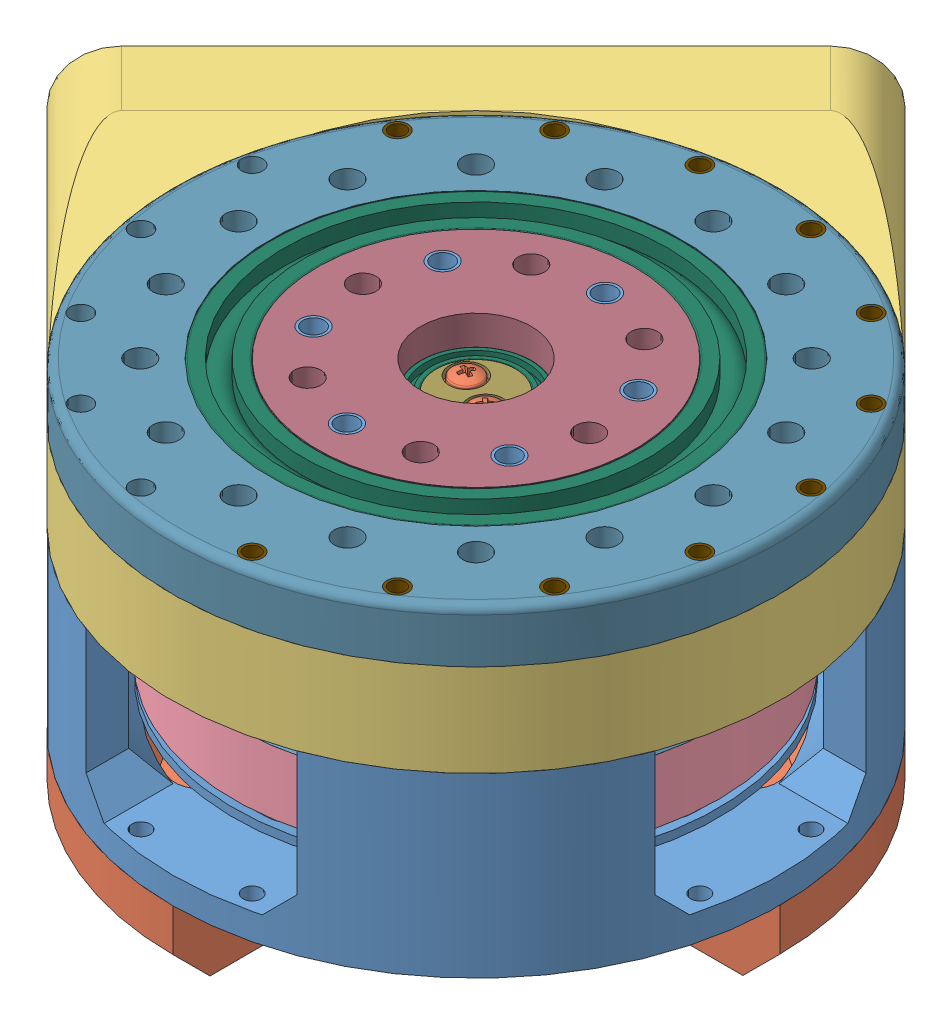
SolidWorks assembly Cycloidal_v2, configuration Default. Lengths in mm.
Overall size (173.24 87.5 173.24).
358 component instances, 93 part files, 154 mates.
Components (placement in the parent):
- motor-X83008S.stp-1: motor-X83008S.stp [Default] at (86.1463 89.8915 109.2516) x (-0.980342 0 -0.197304) z (0 -1 0) size (114.7 114.7 37.62)
  - base.stp-1: base.stp [Default] at (42.0794 12.0269 46.7342) size (91.6 91.6 15.61)
  - stator.stp-1: stator.stp [Default] at (42.0794 12.0269 33.1342) x (0.08493 -0.996387 0) z (0 0 1) size (83 83 8)
  - coil.stp-1: coil.stp [Default] at (39.5332 41.8984 37.1342) x (0.996387 0.08493 0) z (-0.08493 0.996387 0) size (4.4 10.2 10.5)
  - coil.stp-2: coil.stp [Default] at (34.3848 41.0025 37.1342) x (0.966502 0.256661 0) z (-0.256661 0.966502 0) size (4.4 10.2 10.5)
  - coil.stp-3: coil.stp [Default] at (29.4701 39.2261 37.1342) x (0.90725 0.420593 0) z (-0.420593 0.90725 0) size (4.4 10.2 10.5)
  - coil.stp-4: coil.stp [Default] at (24.9386 36.6233 37.1342) x (0.820431 0.571745 0) z (-0.571745 0.820431 0) size (4.4 10.2 10.5)
  - coil.stp-5: coil.stp [Default] at (20.9279 33.2732 37.1342) x (0.708685 0.705525 0) z (-0.705525 0.708685 0) size (4.4 10.2 10.5)
  - coil.stp-6: coil.stp [Default] at (17.5599 29.2775 37.1342) x (0.575405 0.817869 0) z (-0.817869 0.575405 0) size (4.4 10.2 10.5)
  - coil.stp-7: coil.stp [Default] at (14.9368 24.7576 37.1342) x (0.424642 0.905361 0) z (-0.905361 0.424642 0) size (4.4 10.2 10.5)
  - coil.stp-8: coil.stp [Default] at (13.1385 19.8509 37.1342) x (0.260976 0.965345 0) z (-0.965345 0.260976 0) size (4.4 10.2 10.5)
  - coil.stp-9: coil.stp [Default] at (12.2196 14.7066 37.1342) x (0.089381 0.995998 0) z (-0.995998 0.089381 0) size (4.4 10.2 10.5)
  - coil.stp-10: coil.stp [Default] at (12.2079 9.4807 37.1342) x (-0.08493 0.996387 0) z (-0.996387 -0.08493 0) size (4.4 10.2 10.5)
  - coil.stp-11: coil.stp [Default] at (13.1039 4.3323 37.1342) x (-0.256661 0.966502 0) z (-0.966502 -0.256661 0) size (4.4 10.2 10.5)
  - coil.stp-12: coil.stp [Default] at (14.8802 -0.5824 37.1342) x (-0.420593 0.90725 0) z (-0.90725 -0.420593 0) size (4.4 10.2 10.5)
  - coil.stp-13: coil.stp [Default] at (17.483 -5.1139 37.1342) x (-0.571745 0.820431 0) z (-0.820431 -0.571745 0) size (4.4 10.2 10.5)
  - coil.stp-14: coil.stp [Default] at (20.8332 -9.1246 37.1342) x (-0.705525 0.708685 0) z (-0.708685 -0.705525 0) size (4.4 10.2 10.5)
  - coil.stp-15: coil.stp [Default] at (24.8289 -12.4926 37.1342) x (-0.817869 0.575405 0) z (-0.575405 -0.817869 0) size (4.4 10.2 10.5)
  - coil.stp-16: coil.stp [Default] at (29.3487 -15.1157 37.1342) x (-0.905361 0.424642 0) z (-0.424642 -0.905361 0) size (4.4 10.2 10.5)
  - coil.stp-17: coil.stp [Default] at (34.2554 -16.914 37.1342) x (-0.965345 0.260976 0) z (-0.260976 -0.965345 0) size (4.4 10.2 10.5)
  - coil.stp-18: coil.stp [Default] at (39.3998 -17.8329 37.1342) x (-0.995998 0.089381 0) z (-0.089381 -0.995998 0) size (4.4 10.2 10.5)
  - coil.stp-19: coil.stp [Default] at (44.6256 -17.8446 37.1342) x (-0.996387 -0.08493 0) z (0.08493 -0.996387 0) size (4.4 10.2 10.5)
  - coil.stp-20: coil.stp [Default] at (49.7741 -16.9486 37.1342) x (-0.966502 -0.256661 0) z (0.256661 -0.966502 0) size (4.4 10.2 10.5)
  - coil.stp-21: coil.stp [Default] at (54.6887 -15.1723 37.1342) x (-0.90725 -0.420593 0) z (0.420593 -0.90725 0) size (4.4 10.2 10.5)
  - coil.stp-22: coil.stp [Default] at (59.2202 -12.5695 37.1342) x (-0.820431 -0.571745 0) z (0.571745 -0.820431 0) size (4.4 10.2 10.5)
  - coil.stp-23: coil.stp [Default] at (63.2309 -9.2193 37.1342) x (-0.708685 -0.705525 0) z (0.705525 -0.708685 0) size (4.4 10.2 10.5)
  - coil.stp-24: coil.stp [Default] at (66.599 -5.2236 37.1342) x (-0.575405 -0.817869 0) z (0.817869 -0.575405 0) size (4.4 10.2 10.5)
  - coil.stp-25: coil.stp [Default] at (69.222 -0.7038 37.1342) x (-0.424642 -0.905361 0) z (0.905361 -0.424642 0) size (4.4 10.2 10.5)
  - coil.stp-26: coil.stp [Default] at (71.0203 4.2029 37.1342) x (-0.260976 -0.965345 0) z (0.965345 -0.260976 0) size (4.4 10.2 10.5)
  - coil.stp-27: coil.stp [Default] at (71.9392 9.3473 37.1342) x (-0.089381 -0.995998 0) z (0.995998 -0.089381 0) size (4.4 10.2 10.5)
  - coil.stp-28: coil.stp [Default] at (71.9509 14.5731 37.1342) x (0.08493 -0.996387 0) z (0.996387 0.08493 0) size (4.4 10.2 10.5)
  - coil.stp-29: coil.stp [Default] at (71.055 19.7216 37.1342) x (0.256661 -0.966502 0) z (0.966502 0.256661 0) size (4.4 10.2 10.5)
  - coil.stp-30: coil.stp [Default] at (69.2786 24.6362 37.1342) x (0.420593 -0.90725 0) z (0.90725 0.420593 0) size (4.4 10.2 10.5)
  - coil.stp-31: coil.stp [Default] at (66.6758 29.1677 37.1342) x (0.571745 -0.820431 0) z (0.820431 0.571745 0) size (4.4 10.2 10.5)
  - coil.stp-32: coil.stp [Default] at (63.3257 33.1785 37.1342) x (0.705525 -0.708685 0) z (0.708685 0.705525 0) size (4.4 10.2 10.5)
  - coil.stp-33: coil.stp [Default] at (59.33 36.5465 37.1342) x (0.817869 -0.575405 0) z (0.575405 0.817869 0) size (4.4 10.2 10.5)
  - coil.stp-34: coil.stp [Default] at (54.8101 39.1695 37.1342) x (0.905361 -0.424642 0) z (0.424642 0.905361 0) size (4.4 10.2 10.5)
  - coil.stp-35: coil.stp [Default] at (49.9034 40.9678 37.1342) x (0.965345 -0.260976 0) z (0.260976 0.965345 0) size (4.4 10.2 10.5)
  - coil.stp-36: coil.stp [Default] at (44.759 41.8868 37.1342) x (0.995998 -0.089381 0) z (0.089381 0.995998 0) size (4.4 10.2 10.5)
  - rotor.stp-1: rotor.stp [Default] at (42.0794 12.0269 42.1342) x (-0.293442 0.955977 0) z (0 0 -1) size (91.8 91.8 12)
  - outrunner.stp-1: outrunner.stp [Default] at (42.0794 12.0269 30.1342) x (-0.254711 0.967017 0) z (-0.967017 -0.254711 0) size (91.8 17.01 91.8)
  - screw-mount.stp-1: screw-mount.stp [Default] at (38.1314 27.0157 27.1342) x (1 0 0) z (0 0 -1) size (7 7 6.5)
  - screw-mount.stp-2: screw-mount.stp [Default] at (27.0906 8.0789 27.1342) x (1 0 0) z (0 0 -1) size (7 7 6.5)
  - screw-mount.stp-3: screw-mount.stp [Default] at (57.0682 15.9749 27.1342) x (1 0 0) z (0 0 -1) size (7 7 6.5)
  - screw-mount.stp-4: screw-mount.stp [Default] at (46.0274 -2.9618 27.1342) x (1 0 0) z (0 0 -1) size (7 7 6.5)
  - 6702ZZ-bearing-15x21x4.stp-1: 6702ZZ-bearing-15x21x4.stp [Default] at (42.0794 12.0269 43.7342) x (1 0 0) z (0 -1 0) size (21 4 21)
  - 6702ZZ-bearing-15x21x4.stp-2: 6702ZZ-bearing-15x21x4.stp [Default] at (42.0794 12.0269 35.1342) x (1 0 0) z (0 1 0) size (21 4 21)
  - shaft.stp-1: shaft.stp [Default] at (42.0794 12.0269 20.1342) size (16 16 31.6)
  - fix-screw.stp-1: fix-screw.stp [Default] at (42.0794 12.0269 51.7342) x (1 0 0) z (0 0 -1) size (19.67 18.96 12.02)
- Base_Plate-1: Base_Plate [Default] at (47.267 69.7573 89.1587) x (0.897752 0 0.4405) z (-0.4405 0 0.897752) size (40 7 40)
- Eccentric_Shaft-1: Eccentric_Shaft [Default] at (31.2562 70.4165 89.8019) x (0.4405 0 -0.897752) z (0.897752 0 0.4405) size (20 15 17)
  - Eccentric_Shaft_bot-1: Eccentric_Shaft_bot [Default] at (7.6302 6.3409 14.0904) size (17 5 17)
  - Eccentric_Shaft_bot-2: Eccentric_Shaft_bot [Default] at (7.6302 11.3409 14.0904) x (-1 0 0) z (0 0 -1) size (17 5 17)
  - Eccentric_Shaft_top-1: Eccentric_Shaft_top [Default] at (7.6302 16.3409 14.0904) x (-1 0 0) z (0 0 -1) size (17 5 17)
- Output_Shaft-1: Output_Shaft [Default] at (47.267 87.2573 89.1587) x (-0.441786 0 -0.89712) z (0.89712 0 -0.441786) size (60 10 60)
- Cover-1: Cover [Default] at (47.267 87.2573 89.1587) x (0.707107 0 -0.707107) z (0.707107 0 0.707107) size (115 10.4 115)
- radial ball bearing_68_iso-39: radial ball bearing_68_iso [ISO 15 RBB - 1860 - 32,SI,NC,32_68] at (47.267 92.2573 89.1587) x (0 1 0) z (0 0 1) size (10 78 78)
- radial ball bearing_68_iso-40: radial ball bearing_68_iso [ISO 15 RBB - 1840 - 32,SI,NC,32_68] at (47.267 73.2573 89.1587) x (0 1 0) z (-0.019534 0 0.999809) size (7 52 52)
- m13_bearing-31: m13_bearing [Default] at (-10.7414 95.4081 67.0593) x (0.227678 0 0.973736) z (0.973736 0 -0.227678) size (13 16 13)
  - m6-1: m6 [Default] at (8.4921 2.5508 14.8914) size (6 16 6)
  - radial ball bearing_68_iso-1: radial ball bearing_68_iso [ISO 15 RBB - 286 - 10,SI,NC,10_68] at (8.4921 16.0508 14.8914) x (0 1 0) z (0 0 1) size (5 13 13)
  - radial ball bearing_68_iso-2: radial ball bearing_68_iso [ISO 15 RBB - 286 - 10,SI,NC,10_68] at (8.4921 11.0508 14.8914) x (0 1 0) z (0 0 1) size (5 13 13)
- m13_bearing-32: m13_bearing [Default] at (-14.1668 95.4081 84.2801) x (0.227678 0 0.973736) z (0.973736 0 -0.227678) size (13 16 13)
  - m6-1: m6 [Default] at (8.4921 2.5508 14.8914) size (6 16 6)
  - radial ball bearing_68_iso-1: radial ball bearing_68_iso [ISO 15 RBB - 286 - 10,SI,NC,10_68] at (8.4921 16.0508 14.8914) x (0 1 0) z (0 0 1) size (5 13 13)
  - radial ball bearing_68_iso-2: radial ball bearing_68_iso [ISO 15 RBB - 286 - 10,SI,NC,10_68] at (8.4921 11.0508 14.8914) x (0 1 0) z (0 0 1) size (5 13 13)
- m13_bearing-34: m13_bearing [Default] at (13.6125 95.5581 125.8547) x (0.227678 0 0.973736) z (0.973736 0 -0.227678) size (13 16 13)
  - m6-1: m6 [Default] at (8.4921 2.5508 14.8914) size (6 16 6)
  - radial ball bearing_68_iso-1: radial ball bearing_68_iso [ISO 15 RBB - 286 - 10,SI,NC,10_68] at (8.4921 16.0508 14.8914) x (0 1 0) z (0 0 1) size (5 13 13)
  - radial ball bearing_68_iso-2: radial ball bearing_68_iso [ISO 15 RBB - 286 - 10,SI,NC,10_68] at (8.4921 11.0508 14.8914) x (0 1 0) z (0 0 1) size (5 13 13)
- m13_bearing-35: m13_bearing [Default] at (-0.9866 95.4081 116.0999) x (0.227678 0 0.973736) z (0.973736 0 -0.227678) size (13 16 13)
  - m6-1: m6 [Default] at (8.4921 2.5508 14.8914) size (6 16 6)
  - radial ball bearing_68_iso-1: radial ball bearing_68_iso [ISO 15 RBB - 286 - 10,SI,NC,10_68] at (8.4921 16.0508 14.8914) x (0 1 0) z (0 0 1) size (5 13 13)
  - radial ball bearing_68_iso-2: radial ball bearing_68_iso [ISO 15 RBB - 286 - 10,SI,NC,10_68] at (8.4921 11.0508 14.8914) x (0 1 0) z (0 0 1) size (5 13 13)
- m13_bearing-36: m13_bearing [Default] at (-10.7414 95.5581 101.5009) x (0.227678 0 0.973736) z (0.973736 0 -0.227678) size (13 16 13)
  - m6-1: m6 [Default] at (8.4921 2.5508 14.8914) size (6 16 6)
  - radial ball bearing_68_iso-1: radial ball bearing_68_iso [ISO 15 RBB - 286 - 10,SI,NC,10_68] at (8.4921 16.0508 14.8914) x (0 1 0) z (0 0 1) size (5 13 13)
  - radial ball bearing_68_iso-2: radial ball bearing_68_iso [ISO 15 RBB - 286 - 10,SI,NC,10_68] at (8.4921 11.0508 14.8914) x (0 1 0) z (0 0 1) size (5 13 13)
- m13_bearing-1: m13_bearing [Default] at (-0.8801 95.4081 62.5627) x (0.736525 0 0.676411) z (0.676411 0 -0.736525) size (13 16 13)
  - m6-1: m6 [Default] at (8.4921 2.5508 14.8914) size (6 16 6)
  - radial ball bearing_68_iso-1: radial ball bearing_68_iso [ISO 15 RBB - 286 - 10,SI,NC,10_68] at (8.4921 16.0508 14.8914) x (0 1 0) z (0 0 1) size (5 13 13)
  - radial ball bearing_68_iso-2: radial ball bearing_68_iso [ISO 15 RBB - 286 - 10,SI,NC,10_68] at (8.4921 11.0508 14.8914) x (0 1 0) z (0 0 1) size (5 13 13)
- m13_bearing-2: m13_bearing [Default] at (48.6831 95.4081 124.0939) x (0.120271 0 0.992741) z (0.992741 0 -0.120271) size (13 16 13)
  - m6-1: m6 [Default] at (8.4921 2.5508 14.8914) size (6 16 6)
  - radial ball bearing_68_iso-1: radial ball bearing_68_iso [ISO 15 RBB - 286 - 10,SI,NC,10_68] at (8.4921 16.0508 14.8914) x (0 1 0) z (0 0 1) size (5 13 13)
  - radial ball bearing_68_iso-2: radial ball bearing_68_iso [ISO 15 RBB - 286 - 10,SI,NC,10_68] at (8.4921 11.0508 14.8914) x (0 1 0) z (0 0 1) size (5 13 13)
- m13_bearing-3: m13_bearing [Default] at (32.7832 95.4081 34.9886) x (-0.046141 0 0.998935) z (0.998935 0 0.046141) size (13 16 13)
  - m6-1: m6 [Default] at (8.4921 2.5508 14.8914) size (6 16 6)
  - radial ball bearing_68_iso-1: radial ball bearing_68_iso [ISO 15 RBB - 286 - 10,SI,NC,10_68] at (8.4921 16.0508 14.8914) x (0 1 0) z (0 0 1) size (5 13 13)
  - radial ball bearing_68_iso-2: radial ball bearing_68_iso [ISO 15 RBB - 286 - 10,SI,NC,10_68] at (8.4921 11.0508 14.8914) x (0 1 0) z (0 0 1) size (5 13 13)
- m13_bearing-4: m13_bearing [Default] at (77.1902 95.4081 81.0003) x (0.022268 0 0.999752) z (0.999752 0 -0.022268) size (13 16 13)
  - m6-1: m6 [Default] at (8.4921 2.5508 14.8914) size (6 16 6)
  - radial ball bearing_68_iso-1: radial ball bearing_68_iso [ISO 15 RBB - 286 - 10,SI,NC,10_68] at (8.4921 16.0508 14.8914) x (0 1 0) z (0 0 1) size (5 13 13)
  - radial ball bearing_68_iso-2: radial ball bearing_68_iso [ISO 15 RBB - 286 - 10,SI,NC,10_68] at (8.4921 11.0508 14.8914) x (0 1 0) z (0 0 1) size (5 13 13)
- m13_bearing-5: m13_bearing [Default] at (73.474 95.4081 98.7828) x (0.059133 0 0.99825) z (0.99825 0 -0.059133) size (13 16 13)
  - m6-1: m6 [Default] at (8.4921 2.5508 14.8914) size (6 16 6)
  - radial ball bearing_68_iso-1: radial ball bearing_68_iso [ISO 15 RBB - 286 - 10,SI,NC,10_68] at (8.4921 16.0508 14.8914) x (0 1 0) z (0 0 1) size (5 13 13)
  - radial ball bearing_68_iso-2: radial ball bearing_68_iso [ISO 15 RBB - 286 - 10,SI,NC,10_68] at (8.4921 11.0508 14.8914) x (0 1 0) z (0 0 1) size (5 13 13)
- m13_bearing-6: m13_bearing [Default] at (12.9248 95.4081 46.7315) x (0.451561 0 0.89224) z (0.89224 0 -0.451561) size (13 16 13)
  - m6-1: m6 [Default] at (8.4921 2.5508 14.8914) size (6 16 6)
  - radial ball bearing_68_iso-1: radial ball bearing_68_iso [ISO 15 RBB - 286 - 10,SI,NC,10_68] at (8.4921 16.0508 14.8914) x (0 1 0) z (0 0 1) size (5 13 13)
  - radial ball bearing_68_iso-2: radial ball bearing_68_iso [ISO 15 RBB - 286 - 10,SI,NC,10_68] at (8.4921 11.0508 14.8914) x (0 1 0) z (0 0 1) size (5 13 13)
- m13_bearing-7: m13_bearing [Default] at (56.6452 95.4081 32.3406) x (-0.545813 0 0.837907) z (0.837907 0 0.545813) size (13 16 13)
  - m6-1: m6 [Default] at (8.4921 2.5508 14.8914) size (6 16 6)
  - radial ball bearing_68_iso-1: radial ball bearing_68_iso [ISO 15 RBB - 286 - 10,SI,NC,10_68] at (8.4921 16.0508 14.8914) x (0 1 0) z (0 0 1) size (5 13 13)
  - radial ball bearing_68_iso-2: radial ball bearing_68_iso [ISO 15 RBB - 286 - 10,SI,NC,10_68] at (8.4921 11.0508 14.8914) x (0 1 0) z (0 0 1) size (5 13 13)
- m13_bearing-8: m13_bearing [Default] at (63.0373 95.4081 51.3153) x (0.158553 0 0.98735) z (0.98735 0 -0.158553) size (13 16 13)
  - m6-1: m6 [Default] at (8.4921 2.5508 14.8914) size (6 16 6)
  - radial ball bearing_68_iso-1: radial ball bearing_68_iso [ISO 15 RBB - 286 - 10,SI,NC,10_68] at (8.4921 16.0508 14.8914) x (0 1 0) z (0 0 1) size (5 13 13)
  - radial ball bearing_68_iso-2: radial ball bearing_68_iso [ISO 15 RBB - 286 - 10,SI,NC,10_68] at (8.4921 11.0508 14.8914) x (0 1 0) z (0 0 1) size (5 13 13)
- m13_bearing-9: m13_bearing [Default] at (83.8577 95.4081 55.5358) x (-0.687134 0 0.72653) z (0.72653 0 0.687134) size (13 16 13)
  - m6-1: m6 [Default] at (8.4921 2.5508 14.8914) size (6 16 6)
  - radial ball bearing_68_iso-1: radial ball bearing_68_iso [ISO 15 RBB - 286 - 10,SI,NC,10_68] at (8.4921 16.0508 14.8914) x (0 1 0) z (0 0 1) size (5 13 13)
  - radial ball bearing_68_iso-2: radial ball bearing_68_iso [ISO 15 RBB - 286 - 10,SI,NC,10_68] at (8.4921 11.0508 14.8914) x (0 1 0) z (0 0 1) size (5 13 13)
- m13_bearing-11: m13_bearing [Default] at (30.1977 95.4081 135.7424) x (0.57351 0 0.819198) z (0.819198 0 -0.57351) size (13 16 13)
  - m6-1: m6 [Default] at (8.4921 2.5508 14.8914) size (6 16 6)
  - radial ball bearing_68_iso-1: radial ball bearing_68_iso [ISO 15 RBB - 286 - 10,SI,NC,10_68] at (8.4921 16.0508 14.8914) x (0 1 0) z (0 0 1) size (5 13 13)
  - radial ball bearing_68_iso-2: radial ball bearing_68_iso [ISO 15 RBB - 286 - 10,SI,NC,10_68] at (8.4921 11.0508 14.8914) x (0 1 0) z (0 0 1) size (5 13 13)
- m13_bearing-12: m13_bearing [Default] at (62.8861 95.4081 115.3744) x (0.184178 0 0.982893) z (0.982893 0 -0.184178) size (13 16 13)
  - m6-1: m6 [Default] at (8.4921 2.5508 14.8914) size (6 16 6)
  - radial ball bearing_68_iso-1: radial ball bearing_68_iso [ISO 15 RBB - 286 - 10,SI,NC,10_68] at (8.4921 16.0508 14.8914) x (0 1 0) z (0 0 1) size (5 13 13)
  - radial ball bearing_68_iso-2: radial ball bearing_68_iso [ISO 15 RBB - 286 - 10,SI,NC,10_68] at (8.4921 11.0508 14.8914) x (0 1 0) z (0 0 1) size (5 13 13)
- socket button head screw_iso-2: socket button head screw_iso [ISO 7380 - M4 x 12 - 12N] at (47.267 67.4573 134.1587) x (0 1 0) z (-0.724148 0 0.689645) size (14.2 7.6 7.6)
- socket button head screw_iso-3: socket button head screw_iso [ISO 7380 - M4 x 12 - 12N] at (15.4472 67.4573 57.3389) x (0 1 0) z (-0.724148 0 0.689645) size (14.2 7.6 7.6)
- socket button head screw_iso-4: socket button head screw_iso [ISO 7380 - M4 x 12 - 12N] at (30.0462 67.4573 47.5841) x (0 1 0) z (-0.724148 0 0.689645) size (14.2 7.6 7.6)
- socket button head screw_iso-5: socket button head screw_iso [ISO 7380 - M4 x 12 - 12N] at (47.267 67.4573 44.1587) x (0 1 0) z (-0.724148 0 0.689645) size (14.2 7.6 7.6)
- socket button head screw_iso-6: socket button head screw_iso [ISO 7380 - M4 x 12 - 12N] at (64.4877 67.4573 47.5841) x (0 1 0) z (-0.724148 0 0.689645) size (14.2 7.6 7.6)
- socket button head screw_iso-8: socket button head screw_iso [ISO 7380 - M4 x 12 - 12N] at (88.8416 67.4573 71.9379) x (0 1 0) z (-0.724148 0 0.689645) size (14.2 7.6 7.6)
- socket button head screw_iso-9: socket button head screw_iso [ISO 7380 - M4 x 12 - 12N] at (92.267 67.4573 89.1587) x (0 1 0) z (-0.724148 0 0.689645) size (14.2 7.6 7.6)
- socket button head screw_iso-10: socket button head screw_iso [ISO 7380 - M4 x 12 - 12N] at (88.8416 67.4573 106.3794) x (0 1 0) z (-0.724148 0 0.689645) size (14.2 7.6 7.6)
- socket button head screw_iso-11: socket button head screw_iso [ISO 7380 - M4 x 12 - 12N] at (79.0868 67.4573 120.9785) x (0 1 0) z (-0.724148 0 0.689645) size (14.2 7.6 7.6)
- M3x4x4.2_brass_insert-2: M3x4x4.2_brass_insert [Default] at (2.3676 97.2573 59.1579) x (-0.680278 0 -0.732954) z (-0.732954 0 0.680278) size (4 4 4)
- M3x4x4.2_brass_insert-3: M3x4x4.2_brass_insert [Default] at (17.2662 97.2573 44.2593) x (-0.509546 0 -0.860444) z (-0.860444 0 0.509546) size (4 4 4)
- M3x4x4.2_brass_insert-6: M3x4x4.2_brass_insert [Default] at (77.2678 97.2573 44.2593) x (-0.680278 0 -0.732954) z (-0.732954 0 0.680278) size (4 4 4)
- M3x4x4.2_brass_insert-8: M3x4x4.2_brass_insert [Default] at (100.2294 93.2573 78.6238) x (-0.970393 0 0.241533) z (-0.241533 0 -0.970393) size (4 4 4)
- M3x4x4.2_brass_insert-14: M3x4x4.2_brass_insert [Default] at (36.7321 97.2573 36.1963) x (0.509546 0 0.860444) z (0.860444 0 -0.509546) size (4 4 4)
- M3x4x4.2_brass_insert-15: M3x4x4.2_brass_insert [Default] at (57.8019 93.2573 36.1963) x (0.897191 0 -0.441644) z (0.441644 0 0.897191) size (4 4 4)
- M3x4x4.2_brass_insert-16: M3x4x4.2_brass_insert [Default] at (92.1663 97.2573 59.1579) x (-0.680278 0 -0.732954) z (-0.732954 0 0.680278) size (4 4 4)
- M3x4x4.2_brass_insert-17: M3x4x4.2_brass_insert [Default] at (100.2294 97.2573 99.6935) x (0.680278 0 0.732954) z (0.732954 0 -0.680278) size (4 4 4)
- M3x4x4.2_brass_insert-19: M3x4x4.2_brass_insert [Default] at (92.1663 97.2573 119.1595) x (0.680278 0 0.732954) z (0.732954 0 -0.680278) size (4 4 4)
- M3x4x4.2_brass_insert-20: M3x4x4.2_brass_insert [Default] at (77.2678 97.2573 134.058) x (0.680278 0 0.732954) z (0.732954 0 -0.680278) size (4 4 4)
- M3x4x4.2_brass_insert-21: M3x4x4.2_brass_insert [Default] at (57.8019 97.2573 142.1211) x (0.680278 0 0.732954) z (0.732954 0 -0.680278) size (4 4 4)
- M4x6x5.5_brass_insert-47: M4x6x5.5_brass_insert [Default] at (5.6924 92.8573 71.9379) x (0.474598 0 0.880203) z (0 1 0) size (5 5 6)
- M4x6x5.5_brass_insert-48: M4x6x5.5_brass_insert [Default] at (2.267 92.8573 89.1587) x (0.260051 0 0.965595) z (0 1 0) size (5 5 6)
- M4x6x5.5_brass_insert-49: M4x6x5.5_brass_insert [Default] at (5.6924 87.0073 106.3794) x (-0.745833 0 0.666133) z (0 -1 0) size (5 5 6)
- M4x6x5.5_brass_insert-50: M4x6x5.5_brass_insert [Default] at (15.4472 86.8573 120.9785) x (-0.745833 0 0.666133) z (0 -1 0) size (5 5 6)
- M4x6x5.5_brass_insert-51: M4x6x5.5_brass_insert [Default] at (30.0462 87.0073 130.7332) x (0.260051 0 -0.965595) z (0 -1 0) size (5 5 6)
- M4x6x5.5_brass_insert-1: M4x6x5.5_brass_insert [Default] at (60.0558 86.633 70.042) x (-0.745833 0 0.666133) z (0 -1 0) size (5 5 6)
- M4x6x5.5_brass_insert-4: M4x6x5.5_brass_insert [Default] at (57.4281 92.633 109.7924) x (0.260051 0 0.965595) z (0 1 0) size (5 5 6)
- M4x6x5.5_brass_insert-5: M4x6x5.5_brass_insert [Default] at (34.4782 92.633 108.2753) x (0.260051 0 0.965595) z (0 1 0) size (5 5 6)
- M4x6x5.5_brass_insert-6: M4x6x5.5_brass_insert [Default] at (24.3171 92.633 87.6415) x (0.252509 0 0.967595) z (0 1 0) size (5 5 6)
- M4x6x5.5_brass_insert-7: M4x6x5.5_brass_insert [Default] at (37.1059 92.633 68.5249) x (0.175665 0 0.98445) z (0 1 0) size (5 5 6)
- M4x6x5.5_brass_insert-8: M4x6x5.5_brass_insert [Default] at (67.9008 97.2573 78.9976) x (0.260051 0 0.965595) z (0 1 0) size (5 5 6)
- M4x6x5.5_brass_insert-9: M4x6x5.5_brass_insert [Default] at (48.7841 97.2573 66.2088) x (0.260051 0 0.965595) z (0 1 0) size (5 5 6)
- M4x6x5.5_brass_insert-10: M4x6x5.5_brass_insert [Default] at (28.1503 97.2573 76.3698) x (0.009651 0 0.999953) z (0 1 0) size (5 5 6)
- M4x6x5.5_brass_insert-11: M4x6x5.5_brass_insert [Default] at (26.6332 97.2573 99.3197) x (0.260051 0 0.965595) z (0 1 0) size (5 5 6)
- M4x6x5.5_brass_insert-13: M4x6x5.5_brass_insert [Default] at (45.7499 97.2573 112.1086) x (0.260051 0 0.965595) z (0 1 0) size (5 5 6)
- M4x6x5.5_brass_insert-14: M4x6x5.5_brass_insert [Default] at (66.3836 97.2573 101.9475) x (0.260051 0 0.965595) z (0 1 0) size (5 5 6)
- M4x6x5.5_brass_insert-15: M4x6x5.5_brass_insert [Default] at (70.2169 92.633 90.6758) x (0.151918 0 0.988393) z (0 1 0) size (5 5 6)
- M4x6x5.5_brass_insert-20: M4x6x5.5_brass_insert [Default] at (64.4877 86.8573 130.7332) x (-0.745833 0 0.666133) z (0 -1 0) size (5 5 6)
- M4x6x5.5_brass_insert-21: M4x6x5.5_brass_insert [Default] at (47.267 86.8573 134.1587) x (-0.745833 0 0.666133) z (0 -1 0) size (5 5 6)
- M4x6x5.5_brass_insert-22: M4x6x5.5_brass_insert [Default] at (15.4472 86.8573 57.3389) x (0.623293 0 0.781988) z (0 -1 0) size (5 5 6)
- M4x6x5.5_brass_insert-23: M4x6x5.5_brass_insert [Default] at (30.0462 86.8573 47.5841) x (0.623293 0 0.781988) z (0 -1 0) size (5 5 6)
- M4x6x5.5_brass_insert-24: M4x6x5.5_brass_insert [Default] at (79.0868 86.8573 120.9785) x (0.541965 0 0.840401) z (0 -1 0) size (5 5 6)
- M4x6x5.5_brass_insert-25: M4x6x5.5_brass_insert [Default] at (88.8416 86.8573 106.3794) x (-0.745833 0 0.666133) z (0 -1 0) size (5 5 6)
- M4x6x5.5_brass_insert-26: M4x6x5.5_brass_insert [Default] at (92.267 86.8573 89.1587) x (-0.745833 0 0.666133) z (0 -1 0) size (5 5 6)
- M4x6x5.5_brass_insert-27: M4x6x5.5_brass_insert [Default] at (88.8416 86.8573 71.9379) x (-0.745833 0 0.666133) z (0 -1 0) size (5 5 6)
- M4x6x5.5_brass_insert-28: M4x6x5.5_brass_insert [Default] at (79.0868 92.8573 57.3389) x (0.260051 0 0.965595) z (0 1 0) size (5 5 6)
- M4x6x5.5_brass_insert-29: M4x6x5.5_brass_insert [Default] at (64.4877 86.8573 47.5841) x (-0.142939 0 0.989731) z (0 -1 0) size (5 5 6)
- M4x6x5.5_brass_insert-31: M4x6x5.5_brass_insert [Default] at (47.267 86.8573 44.1587) x (-0.220341 0 0.975423) z (0 -1 0) size (5 5 6)
- pan cross head_am-1: pan cross head_am [B18.6.7M - M3 x 0.5 x 20 Type I Cross Recessed PHMS --20N] at (50.858 92.6573 90.9207) x (0 -1 0) z (0.748822 0 0.662771) size (22.37 5.6 5.6)
- pan cross head_am-3: pan cross head_am [B18.6.7M - M3 x 0.5 x 20 Type I Cross Recessed PHMS --20N] at (43.676 92.6573 87.3967) x (0 -1 0) z (0.940321 0 0.340288) size (22.37 5.6 5.6)
- M3x4x4.2_brass_insert-22: M3x4x4.2_brass_insert [Default] at (50.858 69.7573 90.9207) x (0.984578 0 -0.174944) z (0.174944 0 0.984578) size (4 4 4)
- M3x4x4.2_brass_insert-23: M3x4x4.2_brass_insert [Default] at (43.676 69.7573 87.3967) x (0.984609 0 -0.174769) z (0.174769 0 0.984609) size (4 4 4)
- pan cross head_am-4: pan cross head_am [B18.6.7M - M3 x 0.5 x 10 Type I Cross Recessed PHMS --10N] at (33.3518 77.6573 82.3309) x (0 -1 0) z (0 0 1) size (12.37 5.6 5.6)
- pan cross head_am-5: pan cross head_am [B18.6.7M - M3 x 0.5 x 10 Type I Cross Recessed PHMS --10N] at (61.1822 77.6573 95.9864) x (0 -1 0) z (0 0 1) size (12.37 5.6 5.6)
- pan cross head_am-6: pan cross head_am [B18.6.7M - M3 x 0.5 x 10 Type I Cross Recessed PHMS --10N] at (40.4392 77.6573 103.0738) x (0 -1 0) z (0 0 1) size (12.37 5.6 5.6)
- pan cross head_am-7: pan cross head_am [B18.6.7M - M3 x 0.5 x 10 Type I Cross Recessed PHMS --10N] at (54.0947 77.6573 75.2435) x (0 -1 0) z (0 0 1) size (12.37 5.6 5.6)
- radial ball bearing_68_iso-44: radial ball bearing_68_iso [ISO 15 RBB - 1715 - 26,SI,NC,26_68] at (47.9277 84.7573 87.812) x (0 1 0) z (-0.714953 0 -0.699173) size (4 21 21)
- radial ball bearing_68_iso-45: radial ball bearing_68_iso [ISO 15 RBB - 1715 - 26,SI,NC,26_68] at (47.267 89.7573 89.1587) x (0 1 0) z (0.999483 0 -0.032163) size (4 21 21)
- radial ball bearing_68_iso-46: radial ball bearing_68_iso [ISO 15 RBB - 1715 - 26,SI,NC,26_68] at (46.6062 79.7573 90.5053) x (0 1 0) z (0.000177 0 1) size (4 21 21)
- socket button head screw_iso-37: socket button head screw_iso [ISO 7380 - M4 x 12 - 12N] at (79.0868 67.4573 57.3389) x (0 1 0) z (-0.709975 0 0.704227) size (14.2 7.6 7.6)
- socket button head screw_iso-38: socket button head screw_iso [ISO 7380 - M4 x 12 - 12N] at (64.4877 67.4573 130.7332) x (0 1 0) z (-0.724148 0 0.689645) size (14.2 7.6 7.6)
- foc-motor-controller.step-1: foc-motor-controller.step [Default] at (47.267 33.7573 89.1587) x (-0.707107 0 -0.707107) z (0 -1 0) size (57.23 50 8.13)
  - RTA0040B.step-1: RTA0040B.step [Default] at (12.5014 -1.6986 1.595) x (-0.707107 -0.707107 0) z (0 0 1) size (6 6 1)
    - FRAME.step-1: FRAME.step [Default] x (1 0 0) z (0 -1 0) size (6 0.2 6)
      - SOLID.step-1: SOLID.step [Default] at origin size (0.4 0.2 0.22)
      - SOLID-0.step-1: SOLID-0.step [Default] at origin size (0.4 0.2 0.22)
      - SOLID-1.step-1: SOLID-1.step [Default] at origin size (0.4 0.2 0.22)
      - SOLID-2.step-1: SOLID-2.step [Default] at origin size (0.4 0.2 0.22)
      - SOLID-3.step-1: SOLID-3.step [Default] at origin size (0.4 0.2 0.22)
      - SOLID-4.step-1: SOLID-4.step [Default] at origin size (0.4 0.2 0.22)
      - SOLID-5.step-1: SOLID-5.step [Default] at origin size (0.4 0.2 0.22)
      - SOLID-6.step-1: SOLID-6.step [Default] at origin size (0.4 0.2 0.22)
      - SOLID-7.step-1: SOLID-7.step [Default] at origin size (0.4 0.2 0.22)
      - SOLID-8.step-1: SOLID-8.step [Default] at origin size (0.4 0.2 0.22)
      - SOLID-9.step-1: SOLID-9.step [Default] at origin size (0.22 0.2 0.4)
      - SOLID-10.step-1: SOLID-10.step [Default] at origin size (0.22 0.2 0.4)
      - SOLID-11.step-1: SOLID-11.step [Default] at origin size (0.22 0.2 0.4)
      - SOLID-12.step-1: SOLID-12.step [Default] at origin size (0.22 0.2 0.4)
      - SOLID-13.step-1: SOLID-13.step [Default] at origin size (0.22 0.2 0.4)
      - SOLID-14.step-1: SOLID-14.step [Default] at origin size (0.22 0.2 0.4)
      - SOLID-15.step-1: SOLID-15.step [Default] at origin size (0.22 0.2 0.4)
      - SOLID-16.step-1: SOLID-16.step [Default] at origin size (0.22 0.2 0.4)
      - SOLID-17.step-1: SOLID-17.step [Default] at origin size (4.15 0.2 4.15)
      - SOLID-18.step-1: SOLID-18.step [Default] at origin size (0.28 0.1 0.28)
      - SOLID-19.step-1: SOLID-19.step [Default] at origin size (0.28 0.1 0.28)
      - SOLID-20.step-1: SOLID-20.step [Default] at origin size (0.28 0.1 0.28)
      - SOLID-21.step-1: SOLID-21.step [Default] at origin size (0.28 0.1 0.28)
      - SOLID-22.step-1: SOLID-22.step [Default] at origin size (0.4 0.2 0.22)
      - SOLID-23.step-1: SOLID-23.step [Default] at origin size (0.4 0.2 0.22)
      - SOLID-24.step-1: SOLID-24.step [Default] at origin size (0.4 0.2 0.22)
      - SOLID-25.step-1: SOLID-25.step [Default] at origin size (0.4 0.2 0.22)
      - SOLID-26.step-1: SOLID-26.step [Default] at origin size (0.4 0.2 0.22)
      - SOLID-27.step-1: SOLID-27.step [Default] at origin size (0.4 0.2 0.22)
      - SOLID-28.step-1: SOLID-28.step [Default] at origin size (0.4 0.2 0.22)
      - SOLID-29.step-1: SOLID-29.step [Default] at origin size (0.4 0.2 0.22)
      - SOLID-30.step-1: SOLID-30.step [Default] at origin size (0.4 0.2 0.22)
      - SOLID-31.step-1: SOLID-31.step [Default] at origin size (0.4 0.2 0.22)
      - SOLID-32.step-1: SOLID-32.step [Default] at origin size (0.22 0.2 0.4)
      - SOLID-33.step-1: SOLID-33.step [Default] at origin size (0.22 0.2 0.4)
      - SOLID-34.step-1: SOLID-34.step [Default] at origin size (0.22 0.2 0.4)
      - SOLID-35.step-1: SOLID-35.step [Default] at origin size (0.22 0.2 0.4)
      - SOLID-36.step-1: SOLID-36.step [Default] at origin size (0.22 0.2 0.4)
      - SOLID-37.step-1: SOLID-37.step [Default] at origin size (0.22 0.2 0.4)
      - SOLID-38.step-1: SOLID-38.step [Default] at origin size (0.22 0.2 0.4)
      - SOLID-39.step-1: SOLID-39.step [Default] at origin size (0.22 0.2 0.4)
      - SOLID-40.step-1: SOLID-40.step [Default] at origin size (0.22 0.2 0.4)
      - SOLID-41.step-1: SOLID-41.step [Default] at origin size (0.22 0.2 0.4)
      - SOLID-42.step-1: SOLID-42.step [Default] at origin size (0.22 0.2 0.4)
      - SOLID-43.step-1: SOLID-43.step [Default] at origin size (0.22 0.2 0.4)
    - BODY.step-1: BODY.step [Default] at (0 0 0.025) x (1 0 0) z (0 -1 0) size (6 0.97 6)
  - Resonator_SMD_Murata_CSTxExxV-3Pin_3.0x1.1mm.step-1: Resonator_SMD_Murata_CSTxExxV-3Pin_3.0x1.1mm.step [Default] at (1.8 -7 1.595) x (0 1 0) z (0 0 1) size (3.2 1.35 0.9)
  - C_0603_1608Metric.step-1: C_0603_1608Metric.step [Default] at (6.2 -16.8 1.595) x (0 -1 0) z (0 0 1) size (1.6 0.8 0.8)
  - R_0603_1608Metric.step-1: R_0603_1608Metric.step [Default] at (11.8 -7.375 1.595) x (0 1 0) z (0 0 1) size (1.6 0.8 0.45)
  - R_0603_1608Metric.step-2: R_0603_1608Metric.step [Default] at (13.8 -16.8 1.595) x (0 1 0) z (0 0 1) size (1.6 0.8 0.45)
  - R_0603_1608Metric.step-3: R_0603_1608Metric.step [Default] at (18.1 -5.36 1.595) size (1.6 0.8 0.45)
  - C_0603_1608Metric.step-2: C_0603_1608Metric.step [Default] at (2.6 -0.5 1.595) x (0 -1 0) z (0 0 1) size (1.6 0.8 0.8)
  - R_0603_1608Metric.step-4: R_0603_1608Metric.step [Default] at (14.6 -11.3 1.595) x (0 1 0) z (0 0 1) size (1.6 0.8 0.45)
  - L_APV_ANR4020.step-1: L_APV_ANR4020.step [Default] at (22.3 -13.7 1.595) x (0 -1 0) z (0 0 1) size (4.02 4 2)
  - C_0603_1608Metric.step-3: C_0603_1608Metric.step [Default] at (0.3 -12.6 1.595) x (-1 0 0) z (0 0 1) size (1.6 0.8 0.8)
  - C_1206_3216Metric.step-1: C_1206_3216Metric.step [Default] at (15.7 11 1.595) x (0 1 0) z (0 0 1) size (3.2 1.6 1.6)
  - C_0603_1608Metric.step-4: C_0603_1608Metric.step [Default] at (0.3 -9.6 1.595) size (1.6 0.8 0.8)
  - R_0603_1608Metric.step-5: R_0603_1608Metric.step [Default] at (12.3 -16.8 1.595) x (0 1 0) z (0 0 1) size (1.6 0.8 0.45)
  - C_0603_1608Metric.step-5: C_0603_1608Metric.step [Default] at (-0.3 -16.6 1.595) x (0 1 0) z (0 0 1) size (1.6 0.8 0.8)
  - R_0603_1608Metric.step-6: R_0603_1608Metric.step [Default] at (10.9 4.1 1.595) size (1.6 0.8 0.45)
  - C_1206_3216Metric.step-2: C_1206_3216Metric.step [Default] at (6.3 11 1.595) x (0 1 0) z (0 0 1) size (3.2 1.6 1.6)
  - XT30PW_2_2_-M.G.B.step-1: XT30PW_2_2_-M.G.B.step [Default] at (-20.5 9.5 1.595) x (0 -1 0) z (-1 0 0) size (15.5 7.1 12.53)
  - R_0603_1608Metric.step-7: R_0603_1608Metric.step [Default] at (0.3 -11.1 1.595) size (1.6 0.8 0.45)
  - C_0603_1608Metric.step-6: C_0603_1608Metric.step [Default] at (19 -0.4 1.595) x (-0.707107 -0.707107 0) z (0 0 1) size (1.6 0.8 0.8)
  - C_1206_3216Metric.step-3: C_1206_3216Metric.step [Default] at (13.3 11 1.595) x (0 1 0) z (0 0 1) size (3.2 1.6 1.6)
  - R_0603_1608Metric.step-8: R_0603_1608Metric.step [Default] at (10.2 -7.375 1.595) x (0 -1 0) z (0 0 1) size (1.6 0.8 0.45)
  - JST_GH_SM08B-GHS-TB_1x08-1MP_P1.25mm_Horizontal.step-1: JST_GH_SM08B-GHS-TB_1x08-1MP_P1.25mm_Horizontal.step [Default] at (10 -22 1.595) size (13.25 4.95 4.25)
  - C_1206_3216Metric.step-4: C_1206_3216Metric.step [Default] at (-12.3 11 1.595) x (0 1 0) z (0 0 1) size (3.2 1.6 1.6)
  - JST_GH_SM06B-GHS-TB_1x06-1MP_P1.25mm_Horizontal.step-1: JST_GH_SM06B-GHS-TB_1x06-1MP_P1.25mm_Horizontal.step [Default] at (-4.3 -22 1.595) size (10.75 4.95 4.25)
  - C_0603_1608Metric.step-7: C_0603_1608Metric.step [Default] at (7.3 -4.5 1.595) x (-1 0 0) z (0 0 1) size (1.6 0.8 0.8)
  - R_0603_1608Metric.step-9: R_0603_1608Metric.step [Default] at (18.1 -3.86 1.595) x (-1 0 0) z (0 0 1) size (1.6 0.8 0.45)
  - C_1206_3216Metric.step-5: C_1206_3216Metric.step [Default] at (22.6794 -1.2206 1.595) x (0.707107 -0.707107 0) z (0 0 1) size (3.2 1.6 1.6)
  - R_Array_Convex_4x0402.step-1: R_Array_Convex_4x0402.step [Default] at (6.8 -2.5 1.595) size (1 2 0.35)
  - R_0603_1608Metric.step-10: R_0603_1608Metric.step [Default] at (7.7 -16.8 1.595) x (0 -1 0) z (0 0 1) size (1.6 0.8 0.45)
  - C_1206_3216Metric.step-6: C_1206_3216Metric.step [Default] at (8.7 11 1.595) x (0 1 0) z (0 0 1) size (3.2 1.6 1.6)
  - C_0603_1608Metric.step-8: C_0603_1608Metric.step [Default] at (16.1 -11.3 1.595) x (0 1 0) z (0 0 1) size (1.6 0.8 0.8)
  - SOT-23-5.step-1: SOT-23-5.step [Default] at (-3.1 -16.6 1.595) x (-1 0 0) z (0 0 1) size (2.8 2.9 1.55)
  - C_0603_1608Metric.step-9: C_0603_1608Metric.step [Default] at (17.8 -13.6 1.595) size (1.6 0.8 0.8)
  - R_0603_1608Metric.step-11: R_0603_1608Metric.step [Default] at (-11.5 -20.3875 1.595) x (0 -1 0) z (0 0 1) size (1.6 0.8 0.45)
  - C_0603_1608Metric.step-10: C_0603_1608Metric.step [Default] at (-12.4 2.3 1.595) x (0 1 0) z (0 0 1) size (1.6 0.8 0.8)
  - C_1206_3216Metric.step-7: C_1206_3216Metric.step [Default] at (18 11 1.595) x (0 1 0) z (0 0 1) size (3.2 1.6 1.6)
  - R_0603_1608Metric.step-12: R_0603_1608Metric.step [Default] at (-10.8105 -14.9971 1.595) x (-1 0 0) z (0 0 1) size (1.6 0.8 0.45)
  - C_0603_1608Metric.step-11: C_0603_1608Metric.step [Default] at (-13.8 -9.4 1.595) x (-1 0 0) z (0 0 1) size (1.6 0.8 0.8)
  - R_0603_1608Metric.step-13: R_0603_1608Metric.step [Default] at (-23.15 -14.5 1.595) x (-1 0 0) z (0 0 1) size (1.6 0.8 0.45)
  - C_0603_1608Metric.step-12: C_0603_1608Metric.step [Default] at (1.1 -0.2 1.595) x (0 1 0) z (0 0 1) size (1.6 0.8 0.8)
  - D_0805_2012Metric.step-1: D_0805_2012Metric.step [Default] at (22.9 -9.6 1.595) x (0 1 0) z (0 0 1) size (2 1.27 0.8)
  - C_0603_1608Metric.step-13: C_0603_1608Metric.step [Default] at (-7.8 3.775 1.595) x (0 -1 0) z (0 0 1) size (1.6 0.8 0.8)
  - R_0603_1608Metric.step-14: R_0603_1608Metric.step [Default] at (-6.4 -12.825 1.595) x (0 1 0) z (0 0 1) size (1.6 0.8 0.45)
  - L_0603_1608Metric.step-1: L_0603_1608Metric.step [Default] at (-10.1 3 1.595) size (1.6 0.8 0.8)
  - C_0603_1608Metric.step-14: C_0603_1608Metric.step [Default] at (17.9 0.7 1.595) x (-0.707107 -0.707107 0) z (0 0 1) size (1.6 0.8 0.8)
  - HVSSOP-10.step-1: HVSSOP-10.step [Default] at (18.6 -9.6 1.595) x (0 -1 0) z (-1 0 0) size (4.9 1.1 3)
  - C_0603_1608Metric.step-15: C_0603_1608Metric.step [Default] at (7.9 4.1 1.595) x (-1 0 0) z (0 0 1) size (1.6 0.8 0.8)
  - C_0603_1608Metric.step-16: C_0603_1608Metric.step [Default] at (21.1 -9.6 1.595) x (0 -1 0) z (0 0 1) size (1.6 0.8 0.8)
  - R_0603_1608Metric.step-15: R_0603_1608Metric.step [Default] at (-10.8105 -11.9971 1.595) x (-1 0 0) z (0 0 1) size (1.6 0.8 0.45)
  - R_0603_1608Metric.step-16: R_0603_1608Metric.step [Default] at (-18.2 -17.4 1.595) size (1.6 0.8 0.45)
  - C_1206_3216Metric.step-8: C_1206_3216Metric.step [Default] at (-3 11 1.595) x (0 1 0) z (0 0 1) size (3.2 1.6 1.6)
  - R_0603_1608Metric.step-17: R_0603_1608Metric.step [Default] at (-16.9 -20.4 1.595) x (0 -1 0) z (0 0 1) size (1.6 0.8 0.45)
  - R_0603_1608Metric.step-18: R_0603_1608Metric.step [Default] at (-13.3 -20.3875 1.595) x (0 -1 0) z (0 0 1) size (1.6 0.8 0.45)
  - R_0603_1608Metric.step-19: R_0603_1608Metric.step [Default] at (-15.1 -20.3875 1.595) x (0 -1 0) z (0 0 1) size (1.6 0.8 0.45)
  - C_0603_1608Metric.step-17: C_0603_1608Metric.step [Default] at (15.5 -14.4 1.595) x (0 -1 0) z (0 0 1) size (1.6 0.8 0.8)
  - LED_0603_1608Metric.step-1: LED_0603_1608Metric.step [Default] at (-11.5 -23.3875 1.595) x (0 1 0) z (0 0 1) size (1.6 0.8 1.1)
  - C_0805_2012Metric.step-1: C_0805_2012Metric.step [Default] at (19.95 -17 1.595) size (2 1.25 1.25)
  - D_SMB.step-1: D_SMB.step [Default] at (-16.5 11.208 1.595) x (0 -1 0) z (0 0 1) size (5.3 3.55 2.15)
  - C_1206_3216Metric.step-9: C_1206_3216Metric.step [Default] at (-5.3 11 1.595) x (0 1 0) z (0 0 1) size (3.2 1.6 1.6)
  - XT30PW_2_2_-M.G.B.step-2: XT30PW_2_2_-M.G.B.step [Default] at (-20.5 -6.5 1.595) x (0 -1 0) z (-1 0 0) size (15.5 7.1 12.53)
  - C_1206_3216Metric.step-10: C_1206_3216Metric.step [Default] at (1.7 11 1.595) x (0 1 0) z (0 0 1) size (3.2 1.6 1.6)
  - C_1206_3216Metric.step-11: C_1206_3216Metric.step [Default] at (11 11 1.595) x (0 1 0) z (0 0 1) size (3.2 1.6 1.6)
  - C_0603_1608Metric.step-18: C_0603_1608Metric.step [Default] at (-6.3 3.775 1.595) x (0 -1 0) z (0 0 1) size (1.6 0.8 0.8)
  - C_0603_1608Metric.step-19: C_0603_1608Metric.step [Default] at (16.8686 1.7314 1.595) x (0.707107 0.707107 0) z (0 0 1) size (1.6 0.8 0.8)
  - C_0603_1608Metric.step-20: C_0603_1608Metric.step [Default] at (-15.0105 -11.1 1.595) size (1.6 0.8 0.8)
  - C_1206_3216Metric.step-12: C_1206_3216Metric.step [Default] at (-7.7 11 1.595) x (0 1 0) z (0 0 1) size (3.2 1.6 1.6)
  - C_0603_1608Metric.step-21: C_0603_1608Metric.step [Default] at (-18.2 -15.8 1.595) size (1.6 0.8 0.8)
  - C_0603_1608Metric.step-22: C_0603_1608Metric.step [Default] at (-2.1 -11.3 1.595) x (0 -1 0) z (0 0 1) size (1.6 0.8 0.8)
  - C_0603_1608Metric.step-23: C_0603_1608Metric.step [Default] at (-10.8105 -13.4971 1.595) size (1.6 0.8 0.8)
  - C_1206_3216Metric.step-13: C_1206_3216Metric.step [Default] at (4 11 1.595) x (0 1 0) z (0 0 1) size (3.2 1.6 1.6)
  - R_0603_1608Metric.step-20: R_0603_1608Metric.step [Default] at (16 -17.8 1.595) x (0 1 0) z (0 0 1) size (1.6 0.8 0.45)
  - Texas_S-PVSON-N8.step-1: Texas_S-PVSON-N8.step [Default] at (-14.4105 -13.7 1.595) x (-1 0 0) z (0 0 1) size (3 2.98 0.92)
  - C_1206_3216Metric.step-14: C_1206_3216Metric.step [Default] at (21 -2.9 1.595) x (0.707107 -0.707107 0) z (0 0 1) size (3.2 1.6 1.6)
  - C_0603_1608Metric.step-24: C_0603_1608Metric.step [Default] at (-5.9 -16.6 1.595) x (0 1 0) z (0 0 1) size (1.6 0.8 0.8)
  - C_0603_1608Metric.step-25: C_0603_1608Metric.step [Default] at (-3.1 -14.1 1.595) size (1.6 0.8 0.8)
  - R_0603_1608Metric.step-21: R_0603_1608Metric.step [Default] at (7.2 -7.375 1.595) x (0 -1 0) z (0 0 1) size (1.6 0.8 0.45)
  - C_1206_3216Metric.step-15: C_1206_3216Metric.step [Default] at (-0.7 11 1.595) x (0 1 0) z (0 0 1) size (3.2 1.6 1.6)
  - LQFP-64_10x10mm_P0.5mm.step-1: LQFP-64_10x10mm_P0.5mm.step [Default] at (-7 -4.5 1.595) x (-1 0 0) z (0 0 1) size (12 12 1.5)
  - C_0805_2012Metric.step-2: C_0805_2012Metric.step [Default] at (23.35 -17 1.595) x (-1 0 0) z (0 0 1) size (2 1.25 1.25)
  - C_0603_1608Metric.step-26: C_0603_1608Metric.step [Default] at (10.8 -16.8 1.595) x (0 -1 0) z (0 0 1) size (1.6 0.8 0.8)
  - R_0603_1608Metric.step-22: R_0603_1608Metric.step [Default] at (17.5 -17.8 1.595) x (0 -1 0) z (0 0 1) size (1.6 0.8 0.45)
  - C_1206_3216Metric.step-16: C_1206_3216Metric.step [Default] at (20.3 11 1.595) x (0 1 0) z (0 0 1) size (3.2 1.6 1.6)
  - R_0603_1608Metric.step-23: R_0603_1608Metric.step [Default] at (9.2 -16.8 1.595) x (0 -1 0) z (0 0 1) size (1.6 0.8 0.45)
  - C_1206_3216Metric.step-17: C_1206_3216Metric.step [Default] at (-10 11 1.595) x (0 1 0) z (0 0 1) size (3.2 1.6 1.6)
  - R_0603_1608Metric.step-24: R_0603_1608Metric.step [Default] at (17.8 -15.2 1.595) size (1.6 0.8 0.45)
  - C_1206_3216Metric.step-18: C_1206_3216Metric.step [Default] at (19.9 2.6 1.595) x (-0.707107 0.707107 0) z (0 0 1) size (3.2 1.6 1.6)
  - C_0603_1608Metric.step-27: C_0603_1608Metric.step [Default] at (13.4 -7.375 1.595) x (0 -1 0) z (0 0 1) size (1.6 0.8 0.8)
  - R_0603_1608Metric.step-25: R_0603_1608Metric.step [Default] at (8.7 -7.375 1.595) x (0 -1 0) z (0 0 1) size (1.6 0.8 0.45)
  - PQFN-8-EP_6x5mm_P1.27mm_Generic.step-1: PQFN-8-EP_6x5mm_P1.27mm_Generic.step [Default] at (4.9 14.4 -0.085) x (0 1 0) z (0 0 -1) size (6.15 5.15 1.09)
  - C_0805_2012Metric.step-3: C_0805_2012Metric.step [Default] at (-3 8.9 -0.085) x (0 1 0) z (0 0 -1) size (2 1.25 1.25)
  - C_0603_1608Metric.step-28: C_0603_1608Metric.step [Default] at (1.5 -4.3 -0.085) x (0 1 0) z (0 0 -1) size (1.6 0.8 0.8)
  - R_2512_6332Metric.step-1: R_2512_6332Metric.step [Default] at (2.1 8.6 -0.085) x (-1 0 0) z (0 0 -1) size (6.3 3.2 0.6)
  - C_0805_2012Metric.step-4: C_0805_2012Metric.step [Default] at (18.8 8.9 -0.085) x (0 1 0) z (0 0 -1) size (2 1.25 1.25)
  - C_0805_2012Metric.step-5: C_0805_2012Metric.step [Default] at (-5.2 8.901 -0.085) x (0 1 0) z (0 0 -1) size (2 1.25 1.25)
  - PQFN-8-EP_6x5mm_P1.27mm_Generic.step-2: PQFN-8-EP_6x5mm_P1.27mm_Generic.step [Default] at (16.9 14.6 -0.085) x (0 -1 0) z (0 0 -1) size (6.15 5.15 1.09)
  - PQFN-8-EP_6x5mm_P1.27mm_Generic.step-3: PQFN-8-EP_6x5mm_P1.27mm_Generic.step [Default] at (-1.1 14.6 -0.085) x (0 -1 0) z (0 0 -1) size (6.15 5.15 1.09)
  - R_0603_1608Metric.step-26: R_0603_1608Metric.step [Default] at (8.2 8.8 -0.085) x (0 1 0) z (0 0 -1) size (1.6 0.8 0.45)
  - R_2512_6332Metric.step-2: R_2512_6332Metric.step [Default] at (-10.3 8.601 -0.085) x (1 0 0) z (0 0 -1) size (6.3 3.2 0.6)
  - TSSOP-16_4.4x5mm_P0.65mm.step-1: TSSOP-16_4.4x5mm_P0.65mm.step [Default] at (0 0 -0.085) x (-1 0 0) z (0 0 -1) size (6.4 5 1.1)
  - C_0603_1608Metric.step-29: C_0603_1608Metric.step [Default] at (0 -4.25 -0.085) x (0 1 0) z (0 0 -1) size (1.6 0.8 0.8)
  - PQFN-8-EP_6x5mm_P1.27mm_Generic.step-4: PQFN-8-EP_6x5mm_P1.27mm_Generic.step [Default] at (10.9 14.4 -0.085) x (0 1 0) z (0 0 -1) size (6.15 5.15 1.09)
  - R_2512_6332Metric.step-3: R_2512_6332Metric.step [Default] at (13.7 8.6 -0.085) x (1 0 0) z (0 0 -1) size (6.3 3.2 0.6)
  - PQFN-8-EP_6x5mm_P1.27mm_Generic.step-5: PQFN-8-EP_6x5mm_P1.27mm_Generic.step [Default] at (-13.1 14.401 -0.085) x (0 1 0) z (0 0 -1) size (6.15 5.15 1.09)
  - C_0603_1608Metric.step-30: C_0603_1608Metric.step [Default] at (-1.5 -4.3 -0.085) x (0 -1 0) z (0 0 -1) size (1.6 0.8 0.8)
  - PQFN-8-EP_6x5mm_P1.27mm_Generic.step-6: PQFN-8-EP_6x5mm_P1.27mm_Generic.step [Default] at (-7.1 14.601 -0.085) x (0 -1 0) z (0 0 -1) size (6.15 5.15 1.09)
  - foc-motor-controller_PCB.step-1: foc-motor-controller_PCB.step [Default] at origin size (50 50 1.51)
